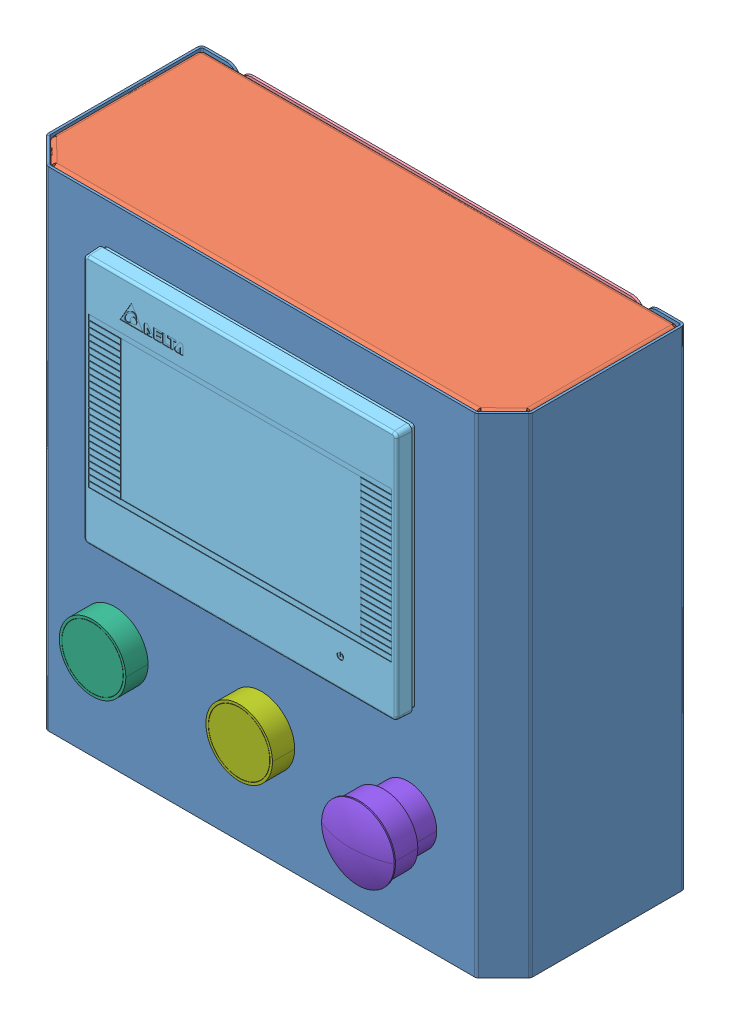
SolidWorks assembly HMI Box Assembly, configuration Default. Lengths in mm.
Overall size (198.22 213.55 100.12).
13 component instances, 9 part files, 0 mates.
Components (placement in the parent):
- HMI Box Assembly.IGS-1: HMI Box Assembly.IGS [Default] at origin size (198.22 213.55 100.12)
  - HMI_Front_Plate.IGS-1: HMI_Front_Plate.IGS [Default] at (87.3329 37.9611 191.9448) size (198.22 200.01 74.62)
  - HMI_Top_Plate.IGS-1: HMI_Top_Plate.IGS [Default] at (87.3329 137.9611 154.6398) size (196.01 22.78 72.01)
  - HMI_Bottom_Plate.IGS-1: HMI_Bottom_Plate.IGS [Default] at (87.3329 -62.0389 154.6398) x (-1 0 0) z (0 0 1) size (196.01 22.78 72.01)
  - HMI_Rear_Plate.IGS-1: HMI_Rear_Plate.IGS [Default] at (87.3329 37.9611 118.6398) size (165.01 200.01 1.01)
  - DOP-B03S211.IGS-1: DOP-B03S211.IGS [Default] at (87.3329 71.9237 200.6448) size (128.64 102.64 40.25)
  - Start PB.IGS-1: Start PB.IGS [Default] at (27.3329 -18.0389 193.0448) size (27.73 27.47 18.37)
  - Stop PB.IGS-1: Stop PB.IGS [Default] at (87.3329 -18.0389 193.0448) size (27.73 27.47 18.37)
  - Emergency PB.IGS-1: Emergency PB.IGS [Default] at (147.3329 -18.0389 201.9448) size (29.74 29.74 48.61)
  - socket button head screw_iso_ISO 7380 - M4 x 8 - 8N.IGS-1: socket button head screw_iso_ISO 7380 - M4 x 8 - 8N.IGS [Default] at (153.6258 129.4611 115.4398) x (0 0 1) z (0.923728 0.383049 0) size (10.24 8.81 7.76)
  - socket button head screw_iso_ISO 7380 - M4 x 8 - 8N.IGS-2: socket button head screw_iso_ISO 7380 - M4 x 8 - 8N.IGS [Default] at (21.04 129.4611 115.4398) x (0 0 1) z (-0.96686 -0.255307 0) size (10.24 8.81 7.76)
  - socket button head screw_iso_ISO 7380 - M4 x 8 - 8N.IGS-3: socket button head screw_iso_ISO 7380 - M4 x 8 - 8N.IGS [Default] at (153.6258 -53.5389 115.4398) x (0 0 1) z (1 0 0) size (10.24 8.81 7.76)
  - socket button head screw_iso_ISO 7380 - M4 x 8 - 8N.IGS-4: socket button head screw_iso_ISO 7380 - M4 x 8 - 8N.IGS [Default] at (21.04 -53.5389 115.4398) x (0 0 1) z (1 0 0) size (10.24 8.81 7.76)
